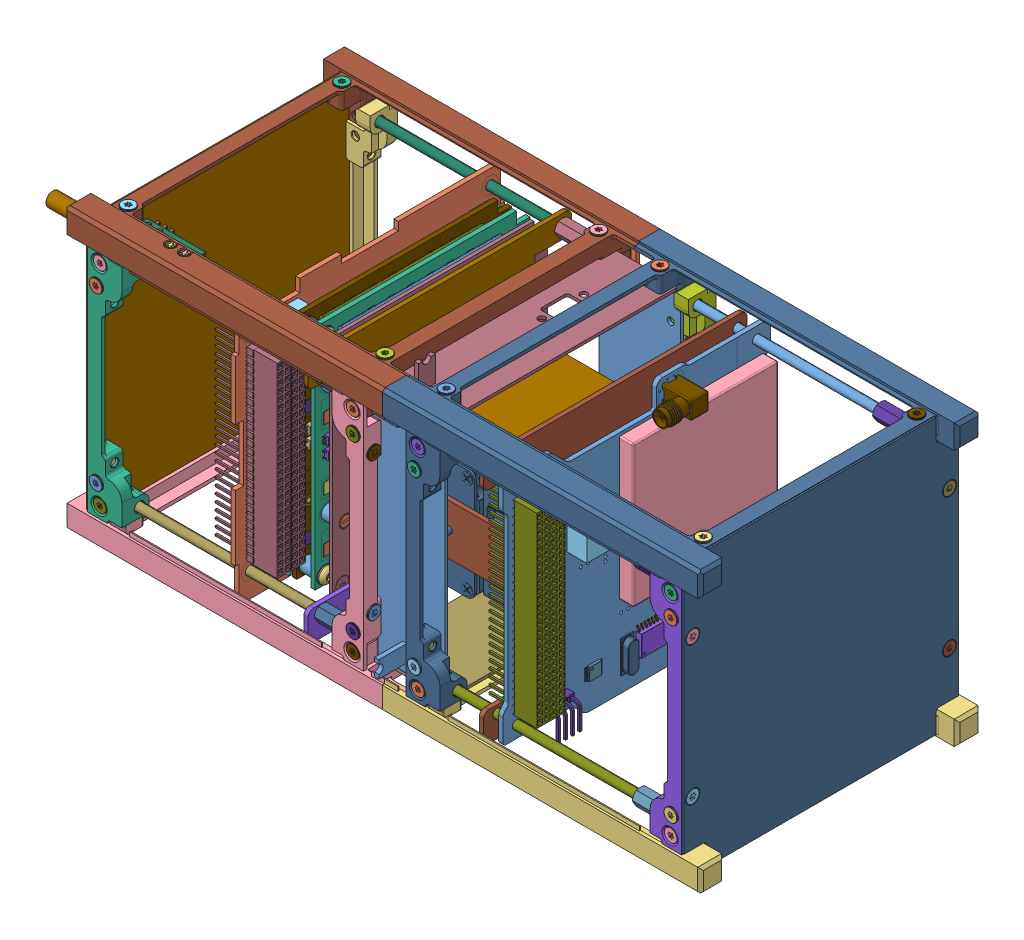
SolidWorks assembly V7A-YONSEI_ONLY_9JAN15, configuration Default. Lengths in mm.
Overall size (235 104.8 105.1).
653 component instances, 272 part files, 0 mates.
Components (placement in the parent):
- ISIS_STR_ASM-1: ISIS_STR_ASM [Default] at (0 -16.675 0) x (0 0 1) z (1 0 0) size (100 100.21 235)
  - PRT0011-1: PRT0011 [Default] at origin size (6 4.7 4.7)
  - PRT0012-1: PRT0012 [Default] at origin size (6 4.7 4.7)
  - PRT0013-1: PRT0013 [Default] at origin size (4.7 4.7 6)
  - PRT0014-1: PRT0014 [Default] at origin size (4.7 4.7 6)
  - PRT0015-1: PRT0015 [Default] at origin size (6 4.7 4.7)
  - PRT0016-1: PRT0016 [Default] at origin size (6 4.7 4.7)
  - PRT0017-1: PRT0017 [Default] at origin size (4.7 4.7 6)
  - PRT0018-1: PRT0018 [Default] at origin size (4.7 4.7 6)
  - PRT0019-1: PRT0019 [Default] at origin size (6 4.7 4.7)
  - PRT0020-1: PRT0020 [Default] at origin size (6 4.7 4.7)
  - PRT0021-1: PRT0021 [Default] at origin size (4.7 4.7 6)
  - PRT0022-1: PRT0022 [Default] at origin size (4.7 4.7 6)
  - PRT0023-1: PRT0023 [Default] at origin size (5.77 5 10)
  - PRT0024-1: PRT0024 [Default] at origin size (5.5 5.5 8)
  - PRT0025-1: PRT0025 [Default] at origin size (3 3 75.8)
  - PRT0026-1: PRT0026 [Default] at origin size (6 4.7 4.7)
  - PRT0027-1: PRT0027 [Default] at origin size (6 4.7 4.7)
  - PRT0028-1: PRT0028 [Default] at origin size (4.7 4.7 6)
  - PRT0029-1: PRT0029 [Default] at origin size (4.7 4.7 6)
  - PRT0030-1: PRT0030 [Default] at origin size (6 4.7 4.7)
  - PRT0031-1: PRT0031 [Default] at origin size (6 4.7 4.7)
  - PRT0032-1: PRT0032 [Default] at origin size (6 4.7 4.7)
  - PRT0033-1: PRT0033 [Default] at origin size (6 4.7 4.7)
  - PRT0034-1: PRT0034 [Default] at origin size (9.7 82.8 12.2)
  - PRT0035-1: PRT0035 [Default] at origin size (5.77 5 10)
  - PRT0108-1: PRT0108 [Default] at origin size (5.5 5.5 8)
  - PRT0109-1: PRT0109 [Default] at origin size (3 3 75.8)
  - PRT0118-1: PRT0118 [Default] at origin size (5.77 5 10)
  - PRT0119-1: PRT0119 [Default] at origin size (5.5 5.5 8)
  - PRT0145-1: PRT0145 [Default] at origin size (3 3 75.8)
  - PRT0146-1: PRT0146 [Default] at origin size (5.77 5 10)
  - PRT0229-1: PRT0229 [Default] at origin size (5.5 5.5 8)
  - PRT0230-1: PRT0230 [Default] at origin size (3 3 75.8)
  - PRT0231-1: PRT0231 [Default] at origin size (6 4.7 4.7)
  - PRT0232-1: PRT0232 [Default] at origin size (6 4.7 4.7)
  - PRT0233-1: PRT0233 [Default] at origin size (6 4.7 4.7)
  - PRT0234-1: PRT0234 [Default] at origin size (6 4.7 4.7)
  - PRT0235-1: PRT0235 [Default] at origin size (9.8 86.8 11.2)
  - PRT0236-1: PRT0236 [Default] at origin size (9.8 86.8 12.2)
  - PRT0237-1: PRT0237 [Default] at origin size (9.7 82.8 11.2)
  - PRT0238-1: PRT0238 [Default] at origin size (6 4.7 4.7)
  - PRT0239-1: PRT0239 [Default] at origin size (6 4.7 4.7)
  - PRT0240-1: PRT0240 [Default] at origin size (4.7 4.7 6)
  - PRT0241-1: PRT0241 [Default] at origin size (4.7 4.7 6)
  - PRT0242-1: PRT0242 [Default] at origin size (6 4.7 4.7)
  - PRT0243-1: PRT0243 [Default] at origin size (6 4.7 4.7)
  - PRT0244-1: PRT0244 [Default] at origin size (4.7 4.7 6)
  - PRT0245-1: PRT0245 [Default] at origin size (4.7 4.7 6)
  - PRT0246-1: PRT0246 [Default] at origin size (6 4.7 4.7)
  - PRT0247-1: PRT0247 [Default] at origin size (6 4.7 4.7)
  - PRT0248-1: PRT0248 [Default] at origin size (4.7 4.7 6)
  - PRT0249-1: PRT0249 [Default] at origin size (4.7 4.7 6)
  - PRT0250-1: PRT0250 [Default] at origin size (5.77 5 10)
  - PRT0251-1: PRT0251 [Default] at origin size (5.5 5.5 8)
  - PRT0252-1: PRT0252 [Default] at origin size (3 3 75.8)
  - PRT0253-1: PRT0253 [Default] at origin size (6 4.7 4.7)
  - PRT0254-1: PRT0254 [Default] at origin size (6 4.7 4.7)
  - PRT0255-1: PRT0255 [Default] at origin size (4.7 4.7 6)
  - PRT0256-1: PRT0256 [Default] at origin size (4.7 4.7 6)
  - PRT0257-1: PRT0257 [Default] at origin size (6 4.7 4.7)
  - PRT0258-1: PRT0258 [Default] at origin size (6 4.7 4.7)
  - PRT0259-1: PRT0259 [Default] at origin size (6 4.7 4.7)
  - PRT0260-1: PRT0260 [Default] at origin size (6 4.7 4.7)
  - PRT0261-1: PRT0261 [Default] at origin size (9.7 82.8 12.2)
  - PRT0262-1: PRT0262 [Default] at origin size (5.77 5 10)
  - PRT0263-1: PRT0263 [Default] at origin size (5.5 5.5 8)
  - PRT0264-1: PRT0264 [Default] at origin size (3 3 75.8)
  - PRT0265-1: PRT0265 [Default] at origin size (5.77 5 10)
  - PRT0266-1: PRT0266 [Default] at origin size (5.5 5.5 8)
  - PRT0267-1: PRT0267 [Default] at origin size (3 3 75.8)
  - PRT0268-1: PRT0268 [Default] at origin size (5.77 5 10)
  - PRT0269-1: PRT0269 [Default] at origin size (5.5 5.5 8)
  - PRT0270-1: PRT0270 [Default] at origin size (3 3 75.8)
  - PRT0271-1: PRT0271 [Default] at origin size (6 4.7 4.7)
  - PRT0272-1: PRT0272 [Default] at origin size (6 4.7 4.7)
  - PRT0273-1: PRT0273 [Default] at origin size (6 4.7 4.7)
  - PRT0274-1: PRT0274 [Default] at origin size (6 4.7 4.7)
  - PRT0275-1: PRT0275 [Default] at origin size (9.8 86.8 11.2)
  - PRT0276-1: PRT0276 [Default] at origin size (9.8 86.8 12.2)
  - PRT0277-1: PRT0277 [Default] at origin size (9.7 82.8 11.2)
  - PRT0278-1: PRT0278 [Default] at origin size (98 98 0.6)
  - PRT0279-1: PRT0279 [Default] at origin size (98 98 0.6)
  - PRT0280-1: PRT0280 [Default] at origin size (4.7 6 4.7)
  - PRT0281-1: PRT0281 [Default] at origin size (4.7 6 4.7)
  - PRT0282-1: PRT0282 [Default] at origin size (4.7 6 4.7)
  - PRT0283-1: PRT0283 [Default] at origin size (4.7 6 4.7)
  - PRT0284-1: PRT0284 [Default] at origin size (4.7 6 4.7)
  - PRT0285-1: PRT0285 [Default] at origin size (4.7 6 4.7)
  - PRT0286-1: PRT0286 [Default] at origin size (4.7 6 4.7)
  - PRT0287-1: PRT0287 [Default] at origin size (4.7 6 4.7)
  - PRT0290-1: PRT0290 [Default] at origin size (3.4 3.4 26)
  - PRT0291-1: PRT0291 [Default] at origin size (5.05 5.05 11.8)
  - PRT0292-1: PRT0292 [Default] at origin size (100 15.4 113.5)
  - PRT0293-1: PRT0293 [Default] at origin size (100 15.5 113.5)
  - PRT0294-1: PRT0294 [Default] at origin size (6.6 2.5 7.5)
  - PRT0295-1: PRT0295 [Default] at origin size (3.2 0.6 6.2)
  - PRT0296-1: PRT0296 [Default] at origin size (7.5 3.11 20.94)
  - PRT0297-1: PRT0297 [Default] at origin size (7.5 0.6 20.94)
  - PRT0298-1: PRT0298 [Default] at origin size (2 1 1.2)
  - PRT0299-1: PRT0299 [Default] at origin size (4.59 2.4 6)
  - PRT0300-1: PRT0300 [Default] at origin size (3.78 3.8 18.32)
  - PRT0301-1: PRT0301 [Default] at origin size (2.4 0.95 2.4)
  - PRT0302-1: PRT0302 [Default] at origin size (2.4 0.95 2.4)
  - PRT0303-1: PRT0303 [Default] at origin size (2.45 0.95 2.45)
  - PRT0304-1: PRT0304 [Default] at origin size (2.45 0.95 2.45)
  - PRT0305-1: PRT0305 [Default] at origin size (3.2 1.3 3.7)
  - PRT0306-1: PRT0306 [Default] at origin size (3.2 1.3 3.7)
  - PRT0307-1: PRT0307 [Default] at origin size (4.7 6 4.7)
  - PRT0308-1: PRT0308 [Default] at origin size (4.7 6 4.7)
  - PRT0309-1: PRT0309 [Default] at origin size (4.7 6 4.7)
  - PRT0310-1: PRT0310 [Default] at origin size (4.7 6 4.7)
  - PRT0311-1: PRT0311 [Default] at origin size (4.7 6 4.7)
  - PRT0312-1: PRT0312 [Default] at origin size (4.7 6 4.7)
  - PRT0313-1: PRT0313 [Default] at origin size (4.7 6 4.7)
  - PRT0314-1: PRT0314 [Default] at origin size (4.7 6 4.7)
  - PRT0317-1: PRT0317 [Default] at origin size (3.4 3.4 26)
  - PRT0318-1: PRT0318 [Default] at origin size (5.05 5.05 11.8)
  - PRT0319-1: PRT0319 [Default] at origin size (100 15.4 113.5)
  - PRT0320-1: PRT0320 [Default] at origin size (100 15.52 113.5)
  - PRT0321-1: PRT0321 [Default] at origin size (6.6 2.5 7.5)
  - PRT0322-1: PRT0322 [Default] at origin size (3.2 0.6 6.2)
  - PRT0323-1: PRT0323 [Default] at origin size (7.5 3.11 20.94)
  - PRT0324-1: PRT0324 [Default] at origin size (7.5 0.6 20.94)
  - PRT0325-1: PRT0325 [Default] at origin size (2 1 1.2)
  - PRT0326-1: PRT0326 [Default] at origin size (4.59 2.4 6)
  - PRT0327-1: PRT0327 [Default] at origin size (3.78 3.8 18.32)
  - PRT0328-1: PRT0328 [Default] at origin size (2.4 0.95 2.4)
  - PRT0329-1: PRT0329 [Default] at origin size (2.4 0.95 2.4)
  - PRT0330-1: PRT0330 [Default] at origin size (2.45 0.95 2.45)
  - PRT0331-1: PRT0331 [Default] at origin size (2.45 0.95 2.45)
  - PRT0332-1: PRT0332 [Default] at origin size (3.2 1.3 3.7)
  - PRT0333-1: PRT0333 [Default] at origin size (3.2 1.3 3.7)
  - PRT0334-1: PRT0334 [Default] at origin size (89 99.8 19.44)
- MOUNT_SHEET_TOTAL_ASM-1: MOUNT_SHEET_TOTAL_ASM [Default] at (94.2438 32.6273 50.75) x (0 1 0) z (0 0 1) size (88.05 65.95 94)
  - MOUNT_BOT-1: MOUNT_BOT [Default] at (0.0477 9.4938 0) size (34.53 43 94)
  - MOUNT_BOT_R-1: MOUNT_BOT_R [Default] at (0.0477 9.4938 0) size (34.53 43 94)
  - RW_-_P015_W_DAMPER__3ASM0463__1-1: RW_-_P015_W_DAMPER__3ASM0463__1 [Default] at (0.0477 -11.307 27.9784) x (1 0.000064 0) z (-0.000064 1 0) size (43.84 22.31 43.84)
  - MOUNT_TOP-1: MOUNT_TOP [Default] at (0 -51.587 -0.0021) x (-1 0 0.000052) z (0.000052 0 1) size (88 61.5 94)
  - RW_-_P015_W_DAMPER__3ASM0463__1-2: RW_-_P015_W_DAMPER__3ASM0463__1 [Default] at (0.0003 -50.9774 6.3179) x (1 0 -0.000052) z (0.000052 0 1) size (43.84 22.31 43.84)
  - RW_-_P015_W_DAMPER__3ASM0463__1-3: RW_-_P015_W_DAMPER__3ASM0463__1 [Default] at (-8.8137 -11.307 -12.68) x (0 -1 0) z (0 0 1) size (43.84 22.31 43.84)
- PRT0010-1: PRT0010 [Default] at (99.05 -9.075 91.15) x (0 0 -1) z (0 -1 0) size (82.5 29 10)
- GOMX-INTERSTAGE-FPP_ASM-1: GOMX-INTERSTAGE-FPP_ASM [Default] at (99.05 75.725 8.85) x (0 0 1) z (0 1 0) size (82.5 29 10)
  - FPP-41_ASM-1: FPP-41_ASM [Default] at origin size (82.5 29 10)
    - FPP-80-1: FPP-80 [Default] at origin size (82.5 29 10)
    - USER_LIBRARY-USB-B-VERT-MINI-1: USER_LIBRARY-USB-B-VERT-MINI [Default] at (26.8339 14.5156 -5.7) x (0 1 0) z (0 0 1) (suppressed, hidden)
- EPS_ASM-1: EPS_ASM [Default] at (-345.0705 -361.6496 49.2336) x (0 1 0.000009) z (0 0.000009 -1) size (90.18 31.69 95.89)
  - ASM0003_ASM-1: ASM0003_ASM [Default] at origin size (90.18 31.69 95.89)
    - PRT0336-1: PRT0336 [Default] at (426.54 417.3615 38.4405) x (0 -1 0) z (0 0 1) size (0.2 6 6)
    - PRT0336-2: PRT0336 [Default] at (362.405 417.3615 38.8225) x (0 -1 0) z (0 0 1) size (0.2 6 6)
    - ASM0004_ASM-1: ASM0004_ASM [Default] at (362.3486 347.5078 -29.4212) size (84.27 11.35 76.64)
      - PRT0337-1: PRT0337 [Default] at (13.1552 69.8437 71.1017) size (1.6 0.9 0.8)
      - PRT0338-1: PRT0338 [Default] at (17.6142 68.2437 64.387) x (0 0 -1) z (-1 0 0) size (1.6 0.55 0.8)
      - PRT0339-1: PRT0339 [Default] at (-5.969 69.8437 65.0687) size (2 0.55 1.25)
      - PRT0340-1: PRT0340 [Default] at (33.4842 67.6187 -0.9016) size (4.5 1.25 3.2)
      - PRT0338-2: PRT0338 [Default] at (44.403 69.8437 66.9107) size (1.6 0.55 0.8)
      - PRT0338-3: PRT0338 [Default] at (19.7732 68.2437 64.387) x (0 0 -1) z (-1 0 0) size (1.6 0.55 0.8)
      - PRT0338-4: PRT0338 [Default] at (46.562 68.2437 66.2757) x (0 0 1) z (1 0 0) size (1.6 0.55 0.8)
      - PRT0338-5: PRT0338 [Default] at (16.8315 68.2437 69.8806) x (0 0 -1) z (-1 0 0) size (1.6 0.55 0.8)
      - PRT0338-6: PRT0338 [Default] at (21.035 68.2437 69.8317) x (0 0 -1) z (-1 0 0) size (1.6 0.55 0.8)
      - ASM0005_ASM-1: ASM0005_ASM [Default] at (10.8213 69.8437 3.9301) x (0 0 1) z (-1 0 0) size (62.81 5 35.56)
        - PRT0341-1: PRT0341 [Default] at origin size (57.81 5 35.56)
        - PRT0342-1: PRT0342 [Default] at origin size (5 0.1 4)
        - PRT0343-1: PRT0343 [Default] at origin size (5 0.1 4)
      - PRT0338-7: PRT0338 [Default] at (-9.1235 68.2437 56.9927) x (1 0 0) z (0 0 -1) size (1.6 0.55 0.8)
      - PRT0338-8: PRT0338 [Default] at (31.703 69.8437 38.3357) size (1.6 0.55 0.8)
      - PRT0338-9: PRT0338 [Default] at (48.467 68.2437 66.2757) x (0 0 1) z (1 0 0) size (1.6 0.55 0.8)
      - PRT0344-1: PRT0344 [Default] at (13.4544 66.7437 0.4732) x (0 -1 0) z (0.000827 0 1) size (3.03 5.56 5.56)
      - PRT0338-10: PRT0338 [Default] at (44.657 68.2437 66.2757) x (0 0 1) z (1 0 0) size (1.6 0.55 0.8)
      - PRT0345-1: PRT0345 [Default] at (41.9699 67.4437 0.9077) x (0 0 -1) z (-1 0 0) size (3.7 1.6 1.6)
      - PRT0338-11: PRT0338 [Default] at (33.8696 68.2437 60.4333) x (0 0 -1) z (-1 0 0) size (1.6 0.55 0.8)
      - PRT0346-1: PRT0346 [Default] at (-360.7506 69.8437 429.8122) x (1 0 0) z (0 1 0) size (84.27 76.64 1.72)
      - PRT0338-12: PRT0338 [Default] at (42.752 68.2437 69.8317) x (0 0 1) z (1 0 0) size (1.6 0.55 0.8)
      - PRT0338-13: PRT0338 [Default] at (44.657 68.2437 69.8317) x (0 0 1) z (1 0 0) size (1.6 0.55 0.8)
      - PRT0338-14: PRT0338 [Default] at (30.6115 69.8437 35.4147) x (0 0 -1) z (1 0 0) size (1.6 0.55 0.8)
      - PRT0345-2: PRT0345 [Default] at (-9.3381 67.4437 52.0887) x (0 0 -1) z (-1 0 0) size (3.7 1.6 1.6)
      - PRT0347-1: PRT0347 [Default] at (31.8644 68.1937 66.8242) x (-1 0 0) z (0 0 -1) size (17.4 5.35 5.5)
      - PRT0337-2: PRT0337 [Default] at (15.4552 68.2437 64.3707) x (0 0 -1) z (-1 0 0) size (1.6 0.9 0.8)
      - PRT0338-15: PRT0338 [Default] at (-9.55 69.8437 61.8847) size (1.6 0.55 0.8)
      - PRT0338-16: PRT0338 [Default] at (14.686 68.2437 69.863) x (0 0 -1) z (-1 0 0) size (1.6 0.55 0.8)
      - ASM0006_ASM-1: ASM0006_ASM [Default] at (31.7757 70.5687 0.0073) size (3.05 1.45 3)
        - PRT0348-1: PRT0348 [Default] at origin size (3.05 1.45 1.75)
        - PRT0349-1: PRT0349 [Default] at origin size (0.4 0.83 0.63)
        - PRT0350-1: PRT0350 [Default] at origin size (0.4 0.83 0.63)
        - PRT0351-1: PRT0351 [Default] at origin size (0.4 0.83 0.63)
        - PRT0352-1: PRT0352 [Default] at origin size (0.4 0.83 0.63)
        - PRT0353-1: PRT0353 [Default] at origin size (0.4 0.83 0.63)
        - PRT0354-1: PRT0354 [Default] at origin size (0.4 0.83 0.63)
      - ASM0006_ASM-2: ASM0006_ASM [Default] at (36.2048 70.5686 -0.0097) x (-0.999553 -0.029894 0.000896) z (-0.000943 0.001563 -0.999998) size (3.05 1.45 3)
        - PRT0348-1: PRT0348 [Default] at origin size (3.05 1.45 1.75)
        - PRT0349-1: PRT0349 [Default] at origin size (0.4 0.83 0.63)
        - PRT0350-1: PRT0350 [Default] at origin size (0.4 0.83 0.63)
        - PRT0351-1: PRT0351 [Default] at origin size (0.4 0.83 0.63)
        - PRT0352-1: PRT0352 [Default] at origin size (0.4 0.83 0.63)
        - PRT0353-1: PRT0353 [Default] at origin size (0.4 0.83 0.63)
        - PRT0354-1: PRT0354 [Default] at origin size (0.4 0.83 0.63)
      - PRT0338-17: PRT0338 [Default] at (32.5293 69.8437 35.4405) x (0 0 -1) z (1 0 0) size (1.6 0.55 0.8)
      - PRT0338-18: PRT0338 [Default] at (19.003 68.2437 69.8317) x (0 0 -1) z (-1 0 0) size (1.6 0.55 0.8)
      - PRT0338-19: PRT0338 [Default] at (12.5406 68.2437 69.7953) x (0 0 -1) z (-1 0 0) size (1.6 0.55 0.8)
      - ASM0005_ASM-2: ASM0005_ASM [Default] at (51.6059 69.8437 3.9301) x (0 0 1) z (-1 0 0) size (62.81 5 35.56)
        - PRT0341-1: PRT0341 [Default] at origin size (57.81 5 35.56)
        - PRT0342-1: PRT0342 [Default] at origin size (5 0.1 4)
        - PRT0343-1: PRT0343 [Default] at origin size (5 0.1 4)
      - PRT0338-20: PRT0338 [Default] at (42.9331 69.8437 69.8649) x (0 0 -1) z (1 0 0) size (1.6 0.55 0.8)
      - PRT0355-1: PRT0355 [Default] at (3.5596 67.4437 -0.2629) x (0 0 -1) z (1 0 0) size (3.15 0.8 6.3)
      - PRT0344-2: PRT0344 [Default] at (53.4544 66.7437 0.4732) x (0 -1 0) z (-0.554303 0 0.832315) size (3.03 5.56 5.56)
      - PRT0338-21: PRT0338 [Default] at (47.832 69.8437 66.9107) size (1.6 0.55 0.8)
      - PRT0338-22: PRT0338 [Default] at (48.467 68.2437 69.8317) x (0 0 1) z (1 0 0) size (1.6 0.55 0.8)
      - PRT0356-1: PRT0356 [Default] at (-9.5164 68.2437 62.3436) x (-0.000827 0 -1) z (-1 0 0.000827) size (6.46 1.2 3)
      - PRT0338-23: PRT0338 [Default] at (42.752 68.2437 66.2757) x (0 0 1) z (1 0 0) size (1.6 0.55 0.8)
      - PRT0338-24: PRT0338 [Default] at (46.562 68.2437 69.8317) x (0 0 1) z (1 0 0) size (1.6 0.55 0.8)
      - PRT0338-25: PRT0338 [Default] at (11.1209 68.2437 62.0624) x (0 0 -1) z (-1 0 0) size (1.6 0.55 0.8)
      - PRT0344-3: PRT0344 [Default] at (7.4544 66.7437 67.4732) x (0 -1 0) z (0.000827 0 1) size (3.03 5.56 5.56)
      - PRT0357-1: PRT0357 [Default] at (-9.6293 70.3937 58.6769) x (-1 0 0) z (0 0 -1) size (3 1.1 2.5)
      - PRT0358-1: PRT0358 [Default] at (15.6729 70.8695 69.1672) x (0 0 -1) z (1 0 0) size (5.01 1.9 6.34)
      - PRT0357-2: PRT0357 [Default] at (31.5849 70.3937 30.9697) x (-1 0 0) z (0 0 -1) size (3 1.1 2.5)
      - PRT0344-4: PRT0344 [Default] at (54.4544 66.7437 67.4732) x (0 -1 0) z (0.000827 0 1) size (3.03 5.56 5.56)
    - PRT0359-1: PRT0359 [Default] at (362.405 415.7515 38.8225) size (5.1 5.01 5.1)
    - PRT0359-2: PRT0359 [Default] at (415.803 422.3515 -28.948) size (5.1 5.01 5.1)
    - PRT0360-1: PRT0360 [Default] at (415.803 423.5515 -28.948) x (0 -1 0) z (0 0 1) size (10 3.8 3.77)
    - PRT0359-3: PRT0359 [Default] at (430.303 415.7515 -29.948) size (5.1 5.01 5.1)
    - PRT0361-1: PRT0361 [Default] at (426.54 419.2115 38.4405) x (0 -1 0) z (0 0 1) size (13.97 5.77 5.75)
    - ASM0007_ASM-1: ASM0007_ASM [Default] at origin size (90.18 23.24 95.89)
      - PRT0362-1: PRT0362 [Default] at (389.1528 402.5515 15.6882) x (0 0 -1) z (-1 0 0) size (7 1.6 5)
      - R0603_ANY-1: R0603_ANY [Default] at (411.005 402.5515 12.2325) x (0 0 -1) z (-1 0 0) size (1.6 0.55 0.8)
      - R0603_ANY-2: R0603_ANY [Default] at (398.093 402.5515 -32.2325) x (0 0 -1) z (-1 0 0) size (1.6 0.55 0.8)
      - R0603_ANY-3: R0603_ANY [Default] at (405.825 402.5515 13.0425) x (-1 0 0) z (0 0 1) size (1.6 0.55 0.8)
      - R0603_ANY-4: R0603_ANY [Default] at (371.825 402.5515 19.9425) x (0 0 -1) z (-1 0 0) size (1.6 0.55 0.8)
      - C0603_ANY-1: C0603_ANY [Default] at (394.7688 401.6515 16.7599) x (0 0 1) z (-1 0 0) size (1.6 0.9 0.8)
      - ASM0008_ASM-1: ASM0008_ASM [Default] at (386.4296 401.8515 -31.1976) x (0 0 -1) z (-1 0 0) size (1.5 1.5 3.6)
        - PRT0363-1: PRT0363 [Default] at origin size (1.5 1.5 1.7)
        - PRT0364-1: PRT0364 [Default] at origin size (1.3 1.3 0.3)
        - PRT0365-1: PRT0365 [Default] at origin size (1.3 1.3 0.4)
        - PRT0366-1: PRT0366 [Default] at origin size (1.3 1.3 0.3)
        - PRT0367-1: PRT0367 [Default] at origin size (1.3 1.3 0.4)
        - PRT0368-1: PRT0368 [Default] at origin size (1.5 1.5 0.5)
      - C0603_ANY-2: C0603_ANY [Default] at (395.4585 401.6515 5.9968) size (1.6 0.9 0.8)
      - PRT0369-1: PRT0369 [Default] at (387.425 406.6915 -42.456) x (0 0 1) z (-1 0 0) size (5.08 23.24 66.55)
      - SO-8_ANY-1: SO-8_ANY [Default] at (418.9388 401.5257 14.6428) x (0 0 -1) z (-1 0 0) size (5.01 1.9 6.34)
      - R0603_ANY-5: R0603_ANY [Default] at (366.225 402.5515 -33.4575) x (-1 0 0) z (0 0 1) size (1.6 0.55 0.8)
      - SOT-23_ANY-1: SOT-23_ANY [Default] at (368.2048 402.0015 20.1191) x (0 0 -1) z (-1 0 0) size (3 1.1 2.5)
      - 3_7V_BATTERY_ANY_ASM-1: 3_7V_BATTERY_ANY_ASM [Default] at (410.3048 404.1515 -25.172) x (0 0 1) z (-1 0 0) size (62.81 5 35.56)
        - NONE-26123-1: NONE-26123 [Default] at origin size (57.81 5 35.56)
        - NONE-26132-1: NONE-26132 [Default] at origin size (5 0.1 4)
        - NONE-26143-1: NONE-26143 [Default] at origin size (5 0.1 4)
      - R0603_ANY-6: R0603_ANY [Default] at (400.252 402.5515 -32.2325) x (0 0 -1) z (-1 0 0) size (1.6 0.55 0.8)
      - C0603_ANY-3: C0603_ANY [Default] at (419.1122 401.6515 7.6332) size (1.6 0.9 0.8)
      - R0603_ANY-7: R0603_ANY [Default] at (351.6397 404.1515 21.3465) x (0 0 -1) z (1 0 0) size (1.6 0.55 0.8)
      - R0603_ANY-8: R0603_ANY [Default] at (387.025 402.5515 -20.9575) x (0 0 -1) z (-1 0 0) size (1.6 0.55 0.8)
      - SOT-23_ANY-2: SOT-23_ANY [Default] at (356.822 402.0015 14.9186) x (1 0 0) z (0 0 -1) size (3 1.1 2.5)
      - PRT0369-2: PRT0369 [Default] at (387.425 406.6915 -37.376) x (0 0 1) z (-1 0 0) size (5.08 23.24 66.55)
      - SO-8_ANY-2: SO-8_ANY [Default] at (363.3251 401.5257 25.9627) x (-1 0 0) z (0 0 1) size (5.01 1.9 6.34)
      - R0603_ANY-9: R0603_ANY [Default] at (411.025 402.5515 8.4525) x (0 0 -1) z (-1 0 0) size (1.6 0.55 0.8)
      - R0603_ANY-10: R0603_ANY [Default] at (354.125 402.5515 27.8425) x (0 0 -1) z (-1 0 0) size (1.6 0.55 0.8)
      - R0603_ANY-11: R0603_ANY [Default] at (357.925 402.5515 19.4425) x (0 0 -1) z (-1 0 0) size (1.6 0.55 0.8)
      - C0603_ANY-4: C0603_ANY [Default] at (414.7449 401.6515 -3.6854) size (1.6 0.9 0.8)
      - R0603_ANY-12: R0603_ANY [Default] at (367.525 402.5515 27.7425) x (0 0 -1) z (-1 0 0) size (1.6 0.55 0.8)
      - R0603_ANY-13: R0603_ANY [Default] at (365.325 402.5515 27.7425) x (0 0 -1) z (-1 0 0) size (1.6 0.55 0.8)
      - R2512_ANY-1: R2512_ANY [Default] at (368.365 401.7515 -22.4432) x (0 0 -1) z (1 0 0) size (3.15 0.8 6.3)
      - SOT-23_ANY-3: SOT-23_ANY [Default] at (406.2499 402.0015 16.2321) x (0 0 -1) z (-1 0 0) size (3 1.1 2.5)
      - PRT0370-1: PRT0370 [Default] at (0 404.1515 402.5515) x (1 0 0) z (0 1 0) size (90.18 95.89 1.72)
      - 3_7V_BATTERY_ANY_ASM-2: 3_7V_BATTERY_ANY_ASM [Default] at (373.2225 404.1515 -25.2198) x (0 0 1) z (-1 0 0) size (62.81 5 35.56)
        - NONE-26123-1: NONE-26123 [Default] at origin size (57.81 5 35.56)
        - NONE-26132-1: NONE-26132 [Default] at origin size (5 0.1 4)
        - NONE-26143-1: NONE-26143 [Default] at origin size (5 0.1 4)
      - SMDC260F-12_ANY-1: SMDC260F-12_ANY [Default] at (381.1322 401.9265 -28.2838) x (0 0 1) z (-1 0 0) size (4.5 1.25 3.2)
      - R0603_ANY-14: R0603_ANY [Default] at (389.425 402.5515 1.5425) x (0 0 -1) z (-1 0 0) size (1.6 0.55 0.8)
      - PRT0371-1: PRT0371 [Default] at (398.2521 402.5015 10.9613) x (0 0 -1) z (-1 0 0) size (7.3 1.84 7.9)
      - PRT0372-1: PRT0372 [Default] at (426.545 409.1515 38.4425) x (0 0 -1) z (1 0 0) size (7 7 7)
      - C0603_ANY-5: C0603_ANY [Default] at (356.3257 401.6515 24.0352) x (0 0 -1) z (1 0 0) size (1.6 0.9 0.8)
      - PRT0372-2: PRT0372 [Default] at (356.885 409.1515 -30.0075) x (0 0 -1) z (1 0 0) size (7 7 7)
      - R0603_ANY-15: R0603_ANY [Default] at (422.125 402.5515 1.0425) x (0 0 -1) z (-1 0 0) size (1.6 0.55 0.8)
      - R0603_ANY-16: R0603_ANY [Default] at (362.325 402.5515 19.4425) x (0 0 -1) z (-1 0 0) size (1.6 0.55 0.8)
      - R0603_ANY-17: R0603_ANY [Default] at (408.565 402.5515 12.2325) x (0 0 -1) z (-1 0 0) size (1.6 0.55 0.8)
      - R0603_ANY-18: R0603_ANY [Default] at (391.325 402.5515 -22.6575) x (0 0 -1) z (-1 0 0) size (1.6 0.55 0.8)
      - PRT0373-1: PRT0373 [Default] at (394.215 404.2015 37.5425) size (17.4 4.15 6.4)
      - ASM0009_ASM-1: ASM0009_ASM [Default] at (396.3269 401.9515 -0.963) x (-1 0 0) z (0 0 1) size (9 1.1 9)
        - PRT0374-1: PRT0374 [Default] at origin size (1.23 0.8 0.22)
        - PRT0375-1: PRT0375 [Default] at origin size (1.23 0.8 0.22)
        - PRT0376-1: PRT0376 [Default] at origin size (1.23 0.8 0.22)
        - PRT0377-1: PRT0377 [Default] at origin size (1.23 0.8 0.22)
        - PRT0378-1: PRT0378 [Default] at origin size (1.23 0.8 0.22)
        - PRT0379-1: PRT0379 [Default] at origin size (1.23 0.8 0.22)
        - PRT0380-1: PRT0380 [Default] at origin size (1.23 0.8 0.22)
        - PRT0381-1: PRT0381 [Default] at origin size (1.23 0.8 0.22)
        - PRT0382-1: PRT0382 [Default] at origin size (1.23 0.8 0.22)
        - PRT0383-1: PRT0383 [Default] at origin size (1.23 0.8 0.22)
        - PRT0384-1: PRT0384 [Default] at origin size (1.23 0.8 0.22)
        - PRT0385-1: PRT0385 [Default] at origin size (1.23 0.8 0.22)
        - PRT0386-1: PRT0386 [Default] at origin size (1.23 0.8 0.22)
        - PRT0387-1: PRT0387 [Default] at origin size (1.23 0.8 0.22)
        - PRT0388-1: PRT0388 [Default] at origin size (1.23 0.8 0.22)
        - PRT0389-1: PRT0389 [Default] at origin size (1.23 0.8 0.22)
        - PRT0390-1: PRT0390 [Default] at origin size (1.23 0.8 0.22)
        - PRT0391-1: PRT0391 [Default] at origin size (1.23 0.8 0.22)
        - PRT0392-1: PRT0392 [Default] at origin size (1.23 0.8 0.22)
        - PRT0393-1: PRT0393 [Default] at origin size (1.23 0.8 0.22)
        - PRT0394-1: PRT0394 [Default] at origin size (1.23 0.8 0.22)
        - PRT0395-1: PRT0395 [Default] at origin size (1.23 0.8 0.22)
        - PRT0396-1: PRT0396 [Default] at origin size (1.23 0.8 0.22)
        - PRT0397-1: PRT0397 [Default] at origin size (1.23 0.8 0.22)
        - PRT0398-1: PRT0398 [Default] at origin size (0.22 0.8 1.23)
        - PRT0399-1: PRT0399 [Default] at origin size (0.22 0.8 1.23)
        - PRT0400-1: PRT0400 [Default] at origin size (0.22 0.8 1.23)
        - PRT0401-1: PRT0401 [Default] at origin size (0.22 0.8 1.23)
        - PRT0402-1: PRT0402 [Default] at origin size (0.22 0.8 1.23)
        - PRT0403-1: PRT0403 [Default] at origin size (0.22 0.8 1.23)
        - PRT0404-1: PRT0404 [Default] at origin size (0.22 0.8 1.23)
        - PRT0405-1: PRT0405 [Default] at origin size (0.22 0.8 1.23)
        - PRT0406-1: PRT0406 [Default] at origin size (0.22 0.8 1.23)
        - PRT0407-1: PRT0407 [Default] at origin size (0.22 0.8 1.23)
        - PRT0408-1: PRT0408 [Default] at origin size (0.22 0.8 1.23)
        - PRT0409-1: PRT0409 [Default] at origin size (0.22 0.8 1.23)
        - PRT0410-1: PRT0410 [Default] at origin size (0.22 0.8 1.23)
        - PRT0411-1: PRT0411 [Default] at origin size (0.22 0.8 1.23)
        - PRT0412-1: PRT0412 [Default] at origin size (0.22 0.8 1.23)
        - PRT0413-1: PRT0413 [Default] at origin size (0.22 0.8 1.23)
        - PRT0414-1: PRT0414 [Default] at origin size (0.22 0.8 1.23)
        - PRT0415-1: PRT0415 [Default] at origin size (0.22 0.8 1.23)
        - PRT0416-1: PRT0416 [Default] at origin size (0.22 0.8 1.23)
        - PRT0417-1: PRT0417 [Default] at origin size (0.22 0.8 1.23)
        - PRT0418-1: PRT0418 [Default] at origin size (0.22 0.8 1.23)
        - PRT0419-1: PRT0419 [Default] at origin size (0.22 0.8 1.23)
        - PRT0420-1: PRT0420 [Default] at origin size (0.22 0.8 1.23)
        - PRT0421-1: PRT0421 [Default] at origin size (0.22 0.8 1.23)
        - PRT0422-1: PRT0422 [Default] at origin size (7 1 7)
      - R0603_ANY-19: R0603_ANY [Default] at (410.855 402.5515 -0.3475) x (0 0 -1) z (-1 0 0) size (1.6 0.55 0.8)
      - R0603_ANY-20: R0603_ANY [Default] at (370.025 402.5515 -33.4575) x (-1 0 0) z (0 0 1) size (1.6 0.55 0.8)
      - SO-8_ANY-3: SO-8_ANY [Default] at (416.5077 401.5257 -1.6713) x (0 0 1) z (1 0 0) size (5.01 1.9 6.34)
      - R0603_ANY-21: R0603_ANY [Default] at (352.825 402.5515 16.0425) x (-1 0 0) z (0 0 1) size (1.6 0.55 0.8)
      - R0603_ANY-22: R0603_ANY [Default] at (352.825 402.5515 18.3425) x (-1 0 0) z (0 0 1) size (1.6 0.55 0.8)
      - R0603_ANY-23: R0603_ANY [Default] at (356.325 402.5515 27.8425) x (0 0 -1) z (-1 0 0) size (1.6 0.55 0.8)
      - R0603_ANY-24: R0603_ANY [Default] at (405.825 402.5515 5.2925) x (-1 0 0) z (0 0 1) size (1.6 0.55 0.8)
      - R0603_ANY-25: R0603_ANY [Default] at (355.825 402.5515 19.4425) x (0 0 -1) z (-1 0 0) size (1.6 0.55 0.8)
      - R0603_ANY-26: R0603_ANY [Default] at (389.125 402.5515 -20.9575) x (0 0 -1) z (-1 0 0) size (1.6 0.55 0.8)
      - SOT-23-5_ANY_ASM-1: SOT-23-5_ANY_ASM [Default] at (390.3459 401.8265 -27.1783) x (1 0 0) z (0 0 -1) size (3.05 1.45 3)
        - NONE-108284-1: NONE-108284 [Default] at origin size (0.4 0.83 0.63)
        - NONE-108285-1: NONE-108285 [Default] at origin size (3.05 1.45 1.75)
        - NONE-108289-1: NONE-108289 [Default] at origin size (0.4 0.83 0.63)
        - NONE-108292-1: NONE-108292 [Default] at origin size (0.4 0.83 0.63)
        - NONE-108294-1: NONE-108294 [Default] at origin size (0.4 0.83 0.63)
        - NONE-108296-1: NONE-108296 [Default] at origin size (0.4 0.83 0.63)
        - NONE-108297-1: NONE-108297 [Default] at origin size (0.4 0.83 0.63)
      - C0603_ANY-6: C0603_ANY [Default] at (365.3256 401.6515 24.0558) x (0 0 -1) z (1 0 0) size (1.6 0.9 0.8)
      - PRT0372-3: PRT0372 [Default] at (430.305 409.1515 -29.9475) x (0 0 -1) z (1 0 0) size (7 7 7)
      - R0603_ANY-27: R0603_ANY [Default] at (351.8913 404.1515 32.8293) size (1.6 0.55 0.8)
      - R0603_ANY-28: R0603_ANY [Default] at (364.525 402.5515 19.4425) x (0 0 -1) z (-1 0 0) size (1.6 0.55 0.8)
      - SOT-23-5_ANY_ASM-2: SOT-23-5_ANY_ASM [Default] at (386.1769 401.8265 -27.1644) x (-1 0 0) z (0 0 1) size (3.05 1.45 3)
        - NONE-108284-1: NONE-108284 [Default] at origin size (0.4 0.83 0.63)
        - NONE-108285-1: NONE-108285 [Default] at origin size (3.05 1.45 1.75)
        - NONE-108289-1: NONE-108289 [Default] at origin size (0.4 0.83 0.63)
        - NONE-108292-1: NONE-108292 [Default] at origin size (0.4 0.83 0.63)
        - NONE-108294-1: NONE-108294 [Default] at origin size (0.4 0.83 0.63)
        - NONE-108296-1: NONE-108296 [Default] at origin size (0.4 0.83 0.63)
        - NONE-108297-1: NONE-108297 [Default] at origin size (0.4 0.83 0.63)
      - PRT0423-1: PRT0423 [Default] at (425.2181 401.0315 12.5431) x (0 0 1) z (-1 0 0) size (2 1.52 1.25)
      - C0603_ANY-7: C0603_ANY [Default] at (413.215 401.6515 12.2177) x (0 0 -1) z (1 0 0) size (1.6 0.9 0.8)
      - R0603_ANY-29: R0603_ANY [Default] at (405.835 402.5515 8.7725) x (-1 0 0) z (0 0 1) size (1.6 0.55 0.8)
      - R0603_ANY-30: R0603_ANY [Default] at (419.025 402.5515 5.4425) x (-1 0 0) z (0 0 1) size (1.6 0.55 0.8)
      - R0603_ANY-31: R0603_ANY [Default] at (405.795 402.5515 10.5925) x (-1 0 0) z (0 0 1) size (1.6 0.55 0.8)
      - PRT0372-4: PRT0372 [Default] at (362.405 409.1515 38.8225) x (0 0 1) z (-1 0 0) size (7 7 7)
      - R0603_ANY-32: R0603_ANY [Default] at (375.762 404.1515 -28.9152) x (0 0 1) z (-1 0 0) size (1.6 0.55 0.8)
      - TSSOP-8_AA__TSSOP-8__ANY-1: TSSOP-8_AA__TSSOP-8__ANY [Default] at (352.0242 404.0015 27.3421) x (0 0 -1) z (1 0 0) size (6.46 1.2 3)
      - R0805_ANY-1: R0805_ANY [Default] at (354.9536 404.1515 36.4614) size (2 0.55 1.25)
      - ASM0008_ASM-2: ASM0008_ASM [Default] at (384.116 401.8515 -23.3928) x (1 0 0) z (0 0 -1) size (1.5 1.5 3.6)
        - PRT0363-1: PRT0363 [Default] at origin size (1.5 1.5 1.7)
        - PRT0364-1: PRT0364 [Default] at origin size (1.3 1.3 0.3)
        - PRT0365-1: PRT0365 [Default] at origin size (1.3 1.3 0.4)
        - PRT0366-1: PRT0366 [Default] at origin size (1.3 1.3 0.3)
        - PRT0367-1: PRT0367 [Default] at origin size (1.3 1.3 0.4)
        - PRT0368-1: PRT0368 [Default] at origin size (1.5 1.5 0.5)
    - PRT0361-2: PRT0361 [Default] at (430.303 419.2115 -29.948) x (0 -1 0) z (-0.991774 0 0.128002) size (13.97 5.77 5.75)
    - PRT0336-3: PRT0336 [Default] at (430.303 417.3615 -29.948) x (0 -1 0) z (0 0 1) size (0.2 6 6)
    - PRT0359-4: PRT0359 [Default] at (426.54 415.7515 38.4405) size (5.1 5.01 5.1)
    - ASM0010_ASM-1: ASM0010_ASM [Default] at (27.76 423.5515 399.502) x (1 0 0) z (0 1 0) size (81.2 76.63 1.3)
      - PRT0424-1: PRT0424 [Default] at origin size (0.84 0.81 0.1)
      - PRT0425-1: PRT0425 [Default] at origin size (81.2 76.63 1.2)
    - PRT0359-5: PRT0359 [Default] at (356.88 415.7515 -30.0115) size (5.1 5.01 5.1)
    - PRT0361-3: PRT0361 [Default] at (362.405 419.2115 38.8225) x (0 -1 0) z (0 0 1) size (13.97 5.77 5.75)
    - ASM0011_ASM-1: ASM0011_ASM [Default] at (362.3486 340.9078 -29.4212) size (84.27 11.35 76.64)
      - R0603_ANY-1: R0603_ANY [Default] at (21.0706 68.2437 69.8317) x (0 0 -1) z (-1 0 0) size (1.6 0.55 0.8)
      - R0603_ANY-2: R0603_ANY [Default] at (16.8849 68.2437 69.8806) x (0 0 -1) z (-1 0 0) size (1.6 0.55 0.8)
      - SOT-23_ANY-1: SOT-23_ANY [Default] at (31.5849 70.3937 30.9697) x (-1 0 0) z (0 0 -1) size (3 1.1 2.5)
      - R0805_ANY-1: R0805_ANY [Default] at (-5.969 69.8437 65.0687) size (2 0.55 1.25)
      - R0603_ANY-3: R0603_ANY [Default] at (46.6663 68.2437 66.2966) x (0 0 1) z (1 0 0) size (1.6 0.55 0.8)
      - MINIMELF_DOMYSLNA_ANY-1: MINIMELF_DOMYSLNA_ANY [Default] at (-9.3381 67.4437 52.0887) x (0 0 -1) z (-1 0 0) size (3.7 1.6 1.6)
      - K3D-KX15-20K3DE-R1_JAE_ANY-1: K3D-KX15-20K3DE-R1_JAE_ANY [Default] at (31.8644 68.1937 66.8242) x (-1 0 0) z (0 0 -1) size (17.4 5.35 5.5)
      - C0603_ANY-1: C0603_ANY [Default] at (13.1552 69.8437 71.1017) size (1.6 0.9 0.8)
      - R0603_ANY-4: R0603_ANY [Default] at (42.9526 69.8437 69.8317) x (0 0 -1) z (1 0 0) size (1.6 0.55 0.8)
      - R0603_ANY-5: R0603_ANY [Default] at (19.8623 68.2437 64.4049) x (0 0 -1) z (-1 0 0) size (1.6 0.55 0.8)
      - SOT-23_ANY-2: SOT-23_ANY [Default] at (-9.6293 70.3937 58.6769) x (-1 0 0) z (0 0 -1) size (3 1.1 2.5)
      - R2512_ANY-1: R2512_ANY [Default] at (3.5596 67.4437 -0.2629) x (0 0 -1) z (1 0 0) size (3.15 0.8 6.3)
      - 3D-13-00246_ANY-1: 3D-13-00246_ANY [Default] at (7.4544 66.7437 67.4732) x (0 -1 0) z (0.000827 0 1) size (3.03 5.56 5.56)
      - R0603_ANY-6: R0603_ANY [Default] at (47.832 69.8437 66.9107) size (1.6 0.55 0.8)
      - R0603_ANY-7: R0603_ANY [Default] at (30.56 69.8437 35.4147) x (0 0 -1) z (1 0 0) size (1.6 0.55 0.8)
      - R0603_ANY-8: R0603_ANY [Default] at (48.5505 68.2437 66.2966) x (0 0 1) z (1 0 0) size (1.6 0.55 0.8)
      - R0603_ANY-9: R0603_ANY [Default] at (33.9113 68.2437 60.4333) x (0 0 -1) z (-1 0 0) size (1.6 0.55 0.8)
      - SMDC260F-12_ANY-1: SMDC260F-12_ANY [Default] at (33.4842 67.6187 -0.9016) size (4.5 1.25 3.2)
      - SOT-23-5_ANY_ASM-1: SOT-23-5_ANY_ASM [Default] at (36.2048 70.5686 -0.0097) x (-0.999553 -0.029894 0.000896) z (-0.000943 0.001563 -0.999998) size (3.05 1.45 3)
        - NONE-108284-1: NONE-108284 [Default] at origin size (0.4 0.83 0.63)
        - NONE-108285-1: NONE-108285 [Default] at origin size (3.05 1.45 1.75)
        - NONE-108289-1: NONE-108289 [Default] at origin size (0.4 0.83 0.63)
        - NONE-108292-1: NONE-108292 [Default] at origin size (0.4 0.83 0.63)
        - NONE-108294-1: NONE-108294 [Default] at origin size (0.4 0.83 0.63)
        - NONE-108296-1: NONE-108296 [Default] at origin size (0.4 0.83 0.63)
        - NONE-108297-1: NONE-108297 [Default] at origin size (0.4 0.83 0.63)
      - R0603_ANY-10: R0603_ANY [Default] at (42.8146 68.2437 66.2757) x (0 0 1) z (1 0 0) size (1.6 0.55 0.8)
      - R0603_ANY-11: R0603_ANY [Default] at (44.7405 68.2437 66.2966) x (0 0 1) z (1 0 0) size (1.6 0.55 0.8)
      - 3_7V_BATTERY_ANY_ASM-1: 3_7V_BATTERY_ANY_ASM [Default] at (10.8213 69.8437 3.8964) x (0 0 1) z (-1 0 0) size (62.81 5 35.56)
        - NONE-26123-1: NONE-26123 [Default] at origin size (57.81 5 35.56)
        - NONE-26132-1: NONE-26132 [Default] at origin size (5 0.1 4)
        - NONE-26143-1: NONE-26143 [Default] at origin size (5 0.1 4)
      - R0603_ANY-12: R0603_ANY [Default] at (32.465 69.8437 35.4147) x (0 0 -1) z (1 0 0) size (1.6 0.55 0.8)
